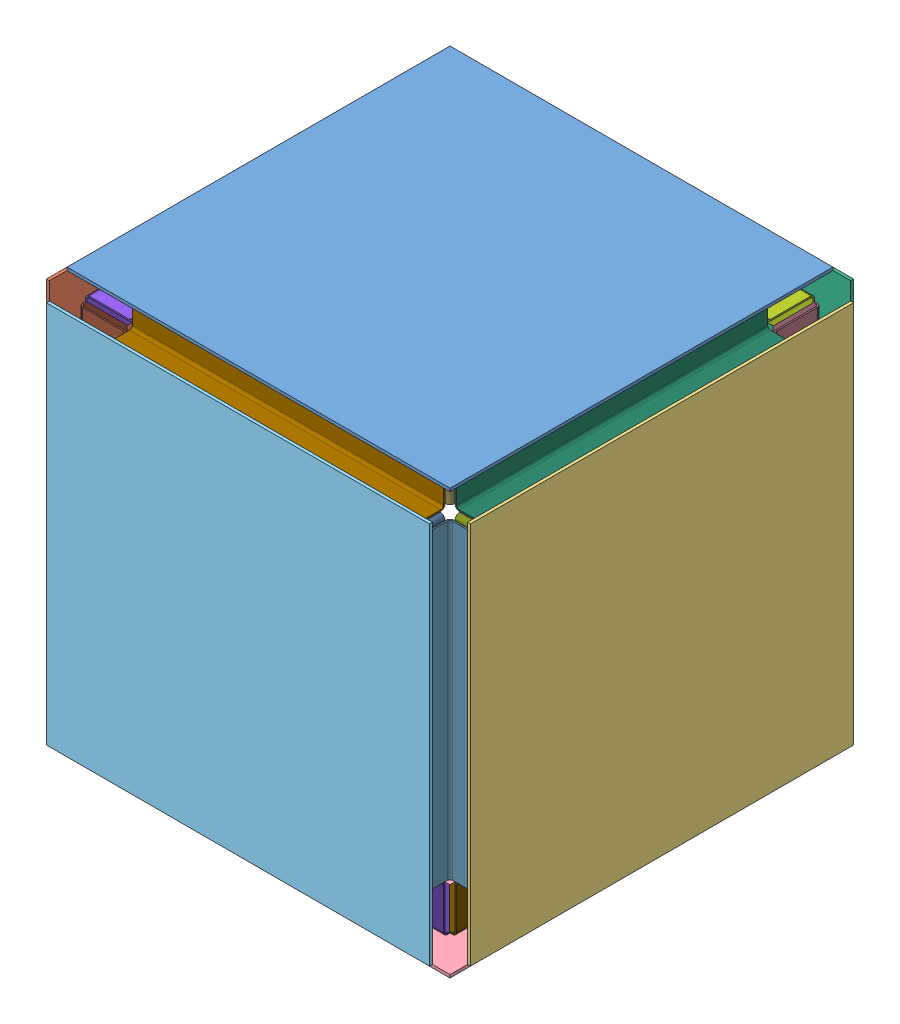
SolidWorks assembly cube_35, configuration cube35. Lengths in mm.
Overall size (229.23 229.23 229.23).
30 component instances, 30 part files, 93 mates.
Components (placement in the parent):
- pr^cube_35-28: pr^cube_35 [cube01] x (-1 0 0) z (0 0 1) size (207.01 1.59 207.01) (virtual)
- pg^cube_35-20: pg^cube_35 [cube01] x (0 -1 0) z (0 0 1) size (207.01 1.59 207.01) (virtual)
- po^cube_35-22: po^cube_35 [cube01] x (0 1 0) z (0 0 1) size (207.01 1.59 207.01) (virtual)
- py^cube_35-21: py^cube_35 [cube01] at origin size (207.01 1.59 207.01) (virtual)
- pc^cube_35-18: pc^cube_35 [cube01] x (-1 0 0) z (0 -1 0) size (207.01 1.59 207.01) (virtual)
- pb^cube_35-21: pb^cube_35 [cube01] x (-1 0 0) z (0 1 0) size (207.01 1.59 207.01) (virtual)
- br1^cube_35-49: br1^cube_35 [Default] at (0 87.63 -87.63) x (0 0 1) z (-1 0 0) size (50.8 50.8 168.15) (virtual)
- br2^cube_35-61: br2^cube_35 [Default] at (-87.63 87.63 0) size (50.8 50.8 168.15) (virtual)
- br3^cube_35-46: br3^cube_35 [Default] at (0 87.63 87.63) x (0 0 -1) z (1 0 0) size (50.8 50.8 168.15) (virtual)
- bg1^cube_35-47: bg1^cube_35 [Default] at (-87.63 -87.63 0) x (0 1 0) z (0 0 1) size (50.8 50.8 168.15) (virtual)
- bg2^cube_35-44: bg2^cube_35 [Default] at (-87.63 0 87.63) x (0 0 -1) z (0 1 0) size (50.8 50.8 168.15) (virtual)
- bg3^cube_35-40: bg3^cube_35 [Default] at (-87.63 0 -87.63) x (0 0 1) z (0 -1 0) size (50.8 50.8 168.15) (virtual)
- bo1^cube_35-42: bo1^cube_35 [Default] at (87.63 0 -87.63) x (0 0 1) z (0 1 0) size (50.8 50.8 168.15) (virtual)
- bo2^cube_35-46: bo2^cube_35 [Default] at (87.63 0 87.63) x (0 0 -1) z (0 -1 0) size (50.8 50.8 168.15) (virtual)
- bo3^cube_35-62: bo3^cube_35 [Default] at (87.63 87.63 0) x (0 -1 0) z (0 0 1) size (50.8 50.8 168.15) (virtual)
- by1^cube_35-41: by1^cube_35 [Default] at (0 -87.63 -87.63) x (0 0 1) z (1 0 0) size (50.8 50.8 168.15) (virtual)
- by2^cube_35-45: by2^cube_35 [Default] at (0 -87.63 87.63) x (0 0 -1) z (-1 0 0) size (50.8 50.8 168.15) (virtual)
- by3^cube_35-48: by3^cube_35 [Default] at (87.63 -87.63 0) x (-1 0 0) z (0 0 1) size (50.8 50.8 168.15) (virtual)
- dr1^cube_35-55: dr1^cube_35 [cube01] at (-112.4246 113.03 0) x (0 -1 0) z (0 0 1) size (26.01 26.01 226.07) (hidden, virtual)
- dr2^cube_35-37: dr2^cube_35 [cube01] at (0 113.03 112.4246) x (0 -1 0) z (1 0 0) size (26.01 26.01 226.07) (hidden, virtual)
- dr3^cube_35-33: dr3^cube_35 [cube01] at (0 113.03 -112.4246) x (0 -1 0) z (-1 0 0) size (26.01 26.01 226.07) (hidden, virtual)
- dg1^cube_35-38: dg1^cube_35 [cube01] at (-113.03 0 112.4246) x (1 0 0) z (0 1 0) size (26.01 26.01 226.07) (hidden, virtual)
- dg2^cube_35-41: dg2^cube_35 [cube01] at (-113.03 -112.4246 0) size (26.01 26.01 226.07) (hidden, virtual)
- dg3^cube_35-34: dg3^cube_35 [cube01] at (-113.03 0 -112.4246) x (1 0 0) z (0 -1 0) size (26.01 26.01 226.07) (hidden, virtual)
- do3^cube_35-47: do3^cube_35 [cube01] at (113.03 112.4246 0) x (-1 0 0) z (0 0 1) size (26.01 26.01 226.07) (hidden, virtual)
- do1^cube_35-36: do1^cube_35 [cube01] at (113.03 0 -112.4246) x (-1 0 0) z (0 1 0) size (26.01 26.01 226.07) (hidden, virtual)
- do2^cube_35-40: do2^cube_35 [cube01] at (113.03 0 112.4246) x (-1 0 0) z (0 -1 0) size (26.01 26.01 226.07) (hidden, virtual)
- dy1^cube_35-35: dy1^cube_35 [cube01] at (0 -113.03 -112.4246) x (0 1 0) z (1 0 0) size (26.01 26.01 226.07) (hidden, virtual)
- dy2^cube_35-39: dy2^cube_35 [cube01] at (0 -113.03 112.4246) x (0 1 0) z (-1 0 0) size (26.01 26.01 226.07) (hidden, virtual)
- dy3^cube_35-42: dy3^cube_35 [cube01] at (112.4246 -113.03 0) x (0 1 0) z (0 0 1) size (26.01 26.01 226.07) (hidden, virtual)
Mates (geometry in assembly coordinates):
- Coincident1: coincident anti-aligned: plane of pr^cube_35-28 through (103.505 113.03 -103.505) normal (0 -1 0); plane of br1^cube_35-49 through (-84.074 113.03 -87.63) normal (0 1 0)
- Coincident2: coincident anti-aligned: plane of pr^cube_35-28 through (103.505 113.03 -103.505) normal (0 -1 0); plane of br2^cube_35-61 through (-87.63 113.03 84.074) normal (0 1 0)
- Coincident3: coincident anti-aligned: plane of pr^cube_35-28 through (103.505 113.03 -103.505) normal (0 -1 0); plane of br3^cube_35-46 through (84.074 113.03 87.63) normal (0 1 0)
- Coincident4: coincident anti-aligned: plane of pr^cube_35-28 through (103.505 113.03 -103.505) normal (0 -1 0); plane of bo3^cube_35-62 through (87.63 113.03 84.074) normal (0 1 0)
- Coincident5: coincident anti-aligned: plane of pr^cube_35-28 through (103.505 113.03 -103.505) normal (0 -1 0); plane of dr3^cube_35-33 through (0 113.03 -225.4546) normal (0 1 0)
- Coincident6: coincident anti-aligned: plane of pr^cube_35-28 through (103.505 113.03 -103.505) normal (0 -1 0); plane of dr1^cube_35-55 through (-225.4546 113.03 0) normal (0 1 0)
- Coincident7: coincident anti-aligned: plane of pr^cube_35-28 through (103.505 113.03 -103.505) normal (0 -1 0); plane of do3^cube_35-47 through (-0.6054 113.03 0) normal (0 1 0)
- Coincident8: coincident anti-aligned: plane of pr^cube_35-28 through (103.505 113.03 -103.505) normal (0 -1 0); plane of dr2^cube_35-37 through (0 113.03 225.4546) normal (0 1 0)
- Coincident34: coincident anti-aligned: plane of pb^cube_35-21 through (103.505 -103.505 -113.03) normal (0 0 1); plane of by1^cube_35-41 through (84.074 -87.63 -113.03) normal (0 0 -1)
- Coincident35: coincident anti-aligned: plane of pb^cube_35-21 through (103.505 -103.505 -113.03) normal (0 0 1); plane of bo1^cube_35-42 through (87.63 84.074 -113.03) normal (0 0 -1)
- Coincident36: coincident anti-aligned: plane of pb^cube_35-21 through (103.505 -103.505 -113.03) normal (0 0 1); plane of br1^cube_35-49 through (-84.074 87.63 -113.03) normal (0 0 -1)
- Coincident37: coincident anti-aligned: plane of pb^cube_35-21 through (103.505 -103.505 -113.03) normal (0 0 1); plane of bg3^cube_35-40 through (-87.63 -84.074 -113.03) normal (0 0 -1)
- Coincident38: coincident anti-aligned: plane of pb^cube_35-21 through (103.505 -103.505 -113.03) normal (0 0 1); plane of dg3^cube_35-34 through (0.6054 0 -113.03) normal (0 0 -1)
- Coincident39: coincident anti-aligned: plane of pb^cube_35-21 through (103.505 -103.505 -113.03) normal (0 0 1); plane of dr3^cube_35-33 through (0 -0.6054 -113.03) normal (0 0 -1)
- Coincident40: coincident anti-aligned: plane of pb^cube_35-21 through (103.505 -103.505 -113.03) normal (0 0 1); plane of do1^cube_35-36 through (-0.6054 0 -113.03) normal (0 0 -1)
- Coincident41: coincident anti-aligned: plane of pb^cube_35-21 through (103.505 -103.505 -113.03) normal (0 0 1); plane of dy1^cube_35-35 through (0 0.6054 -113.03) normal (0 0 -1)
- Coincident42: coincident anti-aligned: plane of pc^cube_35-18 through (103.505 103.505 113.03) normal (0 0 -1); plane of bo2^cube_35-46 through (87.63 -84.074 113.03) normal (0 0 1)
- Coincident43: coincident anti-aligned: plane of pc^cube_35-18 through (103.505 103.505 113.03) normal (0 0 -1); plane of br3^cube_35-46 through (84.074 87.63 113.03) normal (0 0 1)
- Coincident44: coincident anti-aligned: plane of pc^cube_35-18 through (103.505 103.505 113.03) normal (0 0 -1); plane of bg2^cube_35-44 through (-87.63 84.074 113.03) normal (0 0 1)
- Coincident45: coincident anti-aligned: plane of pc^cube_35-18 through (103.505 103.505 113.03) normal (0 0 -1); plane of by2^cube_35-45 through (-84.074 -87.63 113.03) normal (0 0 1)
- Coincident46: coincident anti-aligned: plane of pc^cube_35-18 through (103.505 103.505 113.03) normal (0 0 -1); plane of do2^cube_35-40 through (-0.6054 0 113.03) normal (0 0 1)
- Coincident47: coincident anti-aligned: plane of pc^cube_35-18 through (103.505 103.505 113.03) normal (0 0 -1); plane of dy2^cube_35-39 through (0 0.6054 113.03) normal (0 0 1)
- Coincident48: coincident anti-aligned: plane of pc^cube_35-18 through (103.505 103.505 113.03) normal (0 0 -1); plane of dg1^cube_35-38 through (0.6054 0 113.03) normal (0 0 1)
- Coincident49: coincident anti-aligned: plane of pc^cube_35-18 through (103.505 103.505 113.03) normal (0 0 -1); plane of dr2^cube_35-37 through (0 -0.6054 113.03) normal (0 0 1)
- Coincident50: coincident anti-aligned: plane of pg^cube_35-20 through (-113.03 103.505 -103.505) normal (1 0 0); plane of bg3^cube_35-40 through (-113.03 -84.074 -87.63) normal (-1 0 0)
- Coincident51: coincident anti-aligned: plane of pg^cube_35-20 through (-113.03 103.505 -103.505) normal (1 0 0); plane of bg1^cube_35-47 through (-113.03 -87.63 84.074) normal (-1 0 0)
- Coincident52: coincident anti-aligned: plane of pg^cube_35-20 through (-113.03 103.505 -103.505) normal (1 0 0); plane of bg2^cube_35-44 through (-113.03 84.074 87.63) normal (-1 0 0)
- Coincident53: coincident anti-aligned: plane of pg^cube_35-20 through (-113.03 103.505 -103.505) normal (1 0 0); plane of dr1^cube_35-55 through (-113.03 -0.6054 0) normal (-1 0 0)
- Coincident54: coincident anti-aligned: plane of pg^cube_35-20 through (-113.03 103.505 -103.505) normal (1 0 0); plane of dg3^cube_35-34 through (-113.03 0 -225.4546) normal (-1 0 0)
- Coincident55: coincident anti-aligned: plane of pg^cube_35-20 through (-113.03 103.505 -103.505) normal (1 0 0); plane of dg2^cube_35-41 through (-113.03 -225.4546 0) normal (-1 0 0)
- Coincident56: coincident anti-aligned: plane of pg^cube_35-20 through (-113.03 103.505 -103.505) normal (1 0 0); plane of dg1^cube_35-38 through (-113.03 0 225.4546) normal (-1 0 0)
- Coincident99: coincident anti-aligned: plane of pg^cube_35-20 through (-113.03 103.505 -103.505) normal (1 0 0); plane of br2^cube_35-61 through (-113.03 87.63 84.074) normal (-1 0 0)
- Coincident57: coincident anti-aligned: plane of py^cube_35-21 through (-103.505 -113.03 -103.505) normal (0 1 0); plane of by3^cube_35-48 through (87.63 -113.03 84.074) normal (0 -1 0)
- Coincident58: coincident anti-aligned: plane of py^cube_35-21 through (-103.505 -113.03 -103.505) normal (0 1 0); plane of by2^cube_35-45 through (-84.074 -113.03 87.63) normal (0 -1 0)
- Coincident59: coincident anti-aligned: plane of py^cube_35-21 through (-103.505 -113.03 -103.505) normal (0 1 0); plane of bg1^cube_35-47 through (-87.63 -113.03 84.074) normal (0 -1 0)
- Coincident60: coincident anti-aligned: plane of py^cube_35-21 through (-103.505 -113.03 -103.505) normal (0 1 0); plane of by1^cube_35-41 through (84.074 -113.03 -87.63) normal (0 -1 0)
- Coincident61: coincident anti-aligned: plane of py^cube_35-21 through (-103.505 -113.03 -103.505) normal (0 1 0); plane of dy3^cube_35-42 through (225.4546 -113.03 0) normal (0 -1 0)
- Coincident62: coincident anti-aligned: plane of py^cube_35-21 through (-103.505 -113.03 -103.505) normal (0 1 0); plane of dy2^cube_35-39 through (0 -113.03 225.4546) normal (0 -1 0)
- Coincident63: coincident anti-aligned: plane of py^cube_35-21 through (-103.505 -113.03 -103.505) normal (0 1 0); plane of dg2^cube_35-41 through (0.6054 -113.03 0) normal (0 -1 0)
- Coincident64: coincident anti-aligned: plane of py^cube_35-21 through (-103.505 -113.03 -103.505) normal (0 1 0); plane of dy1^cube_35-35 through (0 -113.03 -225.4546) normal (0 -1 0)
- Coincident65: coincident anti-aligned: plane of po^cube_35-22 through (113.03 -103.505 -103.505) normal (-1 0 0); plane of bo1^cube_35-42 through (113.03 84.074 -87.63) normal (1 0 0)
- Coincident66: coincident anti-aligned: plane of po^cube_35-22 through (113.03 -103.505 -103.505) normal (-1 0 0); plane of by3^cube_35-48 through (113.03 -87.63 84.074) normal (1 0 0)
- Coincident67: coincident anti-aligned: plane of po^cube_35-22 through (113.03 -103.505 -103.505) normal (-1 0 0); plane of bo2^cube_35-46 through (113.03 -84.074 87.63) normal (1 0 0)
- Coincident68: coincident anti-aligned: plane of po^cube_35-22 through (113.03 -103.505 -103.505) normal (-1 0 0); plane of bo3^cube_35-62 through (113.03 87.63 84.074) normal (1 0 0)
- Coincident69: coincident anti-aligned: plane of po^cube_35-22 through (113.03 -103.505 -103.505) normal (-1 0 0); plane of do2^cube_35-40 through (113.03 0 225.4546) normal (1 0 0)
- Coincident70: coincident anti-aligned: plane of po^cube_35-22 through (113.03 -103.505 -103.505) normal (-1 0 0); plane of do3^cube_35-47 through (113.03 225.4546 0) normal (1 0 0)
- Coincident71: coincident anti-aligned: plane of po^cube_35-22 through (113.03 -103.505 -103.505) normal (-1 0 0); plane of do1^cube_35-36 through (113.03 0 -225.4546) normal (1 0 0)
- Coincident72: coincident anti-aligned: plane of po^cube_35-22 through (113.03 -103.505 -103.505) normal (-1 0 0); plane of dy3^cube_35-42 through (113.03 0.6054 0) normal (1 0 0)
- Coincident73: coincident aligned: plane of assembly through (0 0 0) normal (0 0 1); plane of dy3^cube_35-42 through (112.4246 -113.03 0) normal (0 0 1)
- Coincident74: coincident aligned: plane of assembly through (0 0 0) normal (0 0 1); plane of by3^cube_35-48 through (87.63 -87.63 0) normal (0 0 1)
- Coincident75: coincident aligned: plane of assembly through (0 0 0) normal (0 0 1); plane of bo3^cube_35-62 through (87.63 87.63 0) normal (0 0 1)
- Coincident76: coincident aligned: plane of assembly through (0 0 0) normal (0 0 1); plane of do3^cube_35-47 through (113.03 112.4246 0) normal (0 0 1)
- Coincident77: coincident aligned: plane of assembly through (0 0 0) normal (0 0 1); plane of dg2^cube_35-41 through (-113.03 -112.4246 0) normal (0 0 1)
- Coincident78: coincident aligned: plane of assembly through (0 0 0) normal (0 0 1); plane of bg1^cube_35-47 through (-87.63 -87.63 0) normal (0 0 1)
- Coincident79: coincident aligned: plane of assembly through (0 0 0) normal (0 0 1); plane of dr1^cube_35-55 through (-112.4246 113.03 0) normal (0 0 1)
- Coincident80: coincident aligned: plane of assembly through (0 0 0) normal (0 0 1); plane of br2^cube_35-61 through (-87.63 87.63 0) normal (0 0 1)
- Coincident81: coincident aligned: plane of assembly through (0 0 0) normal (0 1 0); plane of bo1^cube_35-42 through (87.63 0 -87.63) normal (0 1 0)
- Coincident82: coincident aligned: plane of assembly through (0 0 0) normal (0 1 0); plane of py^cube_35-21 through (0 0 0) normal (0 1 0)
- Coincident83: coincident aligned: plane of assembly through (0 0 0) normal (0 1 0); plane of do1^cube_35-36 through (113.03 0 -112.4246) normal (0 1 0)
- Coincident84: coincident anti-aligned: plane of assembly through (0 0 0) normal (0 1 0); plane of bg3^cube_35-40 through (-87.63 0 -87.63) normal (0 -1 0)
- Coincident85: coincident anti-aligned: plane of assembly through (0 0 0) normal (0 1 0); plane of dg3^cube_35-34 through (-113.03 0 -112.4246) normal (0 -1 0)
- Coincident86: coincident aligned: plane of assembly through (0 0 0) normal (0 1 0); plane of dg1^cube_35-38 through (-113.03 0 112.4246) normal (0 1 0)
- Coincident87: coincident aligned: plane of assembly through (0 0 0) normal (0 1 0); plane of bg2^cube_35-44 through (-87.63 0 87.63) normal (0 1 0)
- Coincident88: coincident anti-aligned: plane of assembly through (0 0 0) normal (0 1 0); plane of bo2^cube_35-46 through (87.63 0 87.63) normal (0 -1 0)
- Coincident89: coincident anti-aligned: plane of assembly through (0 0 0) normal (0 1 0); plane of do2^cube_35-40 through (113.03 0 112.4246) normal (0 -1 0)
- Coincident90: coincident anti-aligned: plane of assembly through (0 0 0) normal (1 0 0); plane of by2^cube_35-45 through (0 -87.63 87.63) normal (-1 0 0)
- Coincident91: coincident anti-aligned: plane of assembly through (0 0 0) normal (1 0 0); plane of dy2^cube_35-39 through (0 -113.03 112.4246) normal (-1 0 0)
- Coincident92: coincident aligned: plane of assembly through (0 0 0) normal (1 0 0); plane of pg^cube_35-20
- Coincident93: coincident aligned: plane of assembly through (0 0 0) normal (1 0 0); plane of dr2^cube_35-37 through (0 113.03 112.4246) normal (1 0 0)
- Coincident94: coincident aligned: plane of assembly through (0 0 0) normal (1 0 0); plane of br3^cube_35-46 through (0 87.63 87.63) normal (1 0 0)
- Coincident95: coincident anti-aligned: plane of assembly through (0 0 0) normal (1 0 0); plane of dr3^cube_35-33 through (0 113.03 -112.4246) normal (-1 0 0)
- Coincident96: coincident anti-aligned: plane of assembly through (0 0 0) normal (1 0 0); plane of br1^cube_35-49 through (0 87.63 -87.63) normal (-1 0 0)
- Coincident97: coincident aligned: plane of assembly through (0 0 0) normal (1 0 0); plane of by1^cube_35-41 through (0 -87.63 -87.63) normal (1 0 0)
- Coincident98: coincident aligned: plane of assembly through (0 0 0) normal (1 0 0); plane of dy1^cube_35-35 through (0 -113.03 -112.4246) normal (1 0 0)
- Coincident100: coincident anti-aligned: plane of pr^cube_35-28; plane of assembly through (0 0 0) normal (1 0 0)
- Coincident101: coincident aligned: plane of pr^cube_35-28 through (0 0 0) normal (0 0 1); plane of assembly through (0 0 0) normal (0 0 1)
- Coincident102: coincident anti-aligned: plane of pr^cube_35-28; plane of assembly through (0 0 0) normal (0 1 0)
- Coincident106: coincident anti-aligned: plane of pg^cube_35-20; plane of assembly through (0 0 0) normal (0 1 0)
- Coincident107: coincident aligned: plane of pg^cube_35-20; plane of assembly through (0 0 0) normal (1 0 0)
- Coincident108: coincident aligned: plane of pg^cube_35-20 through (0 0 0) normal (0 0 1); plane of assembly through (0 0 0) normal (0 0 1)
- Coincident109: coincident aligned: plane of py^cube_35-21 through (0 0 0) normal (0 0 1); plane of assembly through (0 0 0) normal (0 0 1)
- Coincident110: coincident aligned: plane of py^cube_35-21 through (0 0 0) normal (0 1 0); plane of assembly through (0 0 0) normal (0 1 0)
- Coincident111: coincident aligned: plane of py^cube_35-21 through (0 0 0) normal (1 0 0); plane of assembly through (0 0 0) normal (1 0 0)
- Coincident112: coincident aligned: plane of po^cube_35-22 through (0 0 0) normal (0 0 1); plane of assembly through (0 0 0) normal (0 0 1)
- Coincident113: coincident anti-aligned: plane of po^cube_35-22; plane of assembly through (0 0 0) normal (1 0 0)
- Coincident114: coincident aligned: plane of po^cube_35-22; plane of assembly through (0 0 0) normal (0 1 0)
- Coincident115: coincident anti-aligned: plane of pc^cube_35-18 through (0 0 0) normal (0 -1 0); plane of assembly through (0 0 0) normal (0 1 0)
- Coincident116: coincident anti-aligned: plane of pc^cube_35-18; plane of assembly through (0 0 0) normal (0 0 1)
- Coincident117: coincident anti-aligned: plane of pc^cube_35-18; plane of assembly through (0 0 0) normal (1 0 0)
- Coincident118: coincident aligned: plane of pb^cube_35-21 through (0 0 0) normal (0 1 0); plane of assembly through (0 0 0) normal (0 1 0)
- Coincident119: coincident aligned: plane of pb^cube_35-21; plane of assembly through (0 0 0) normal (0 0 1)
- Coincident120: coincident anti-aligned: line of pb^cube_35-21 through (0.8731 -0.8731 0) axis (0 0 -1); sketch_entity of pr^cube_35-28; plane of pb^cube_35-21 through (103.505 -103.505 -114.6175) normal (0 0 -1); plane of py^cube_35-21 through (-103.505 -114.6175 -103.505) normal (0 -1 0)
- cyan_cut: unknown: unknown of pc^cube_35-18; plane of pc^cube_35-18 through (103.505 103.505 114.6175) normal (0 0 1); plane of pg^cube_35-20 through (-114.6175 103.505 -103.505) normal (-1 0 0); plane of po^cube_35-22 through (114.6175 -103.505 -103.505) normal (1 0 0)
